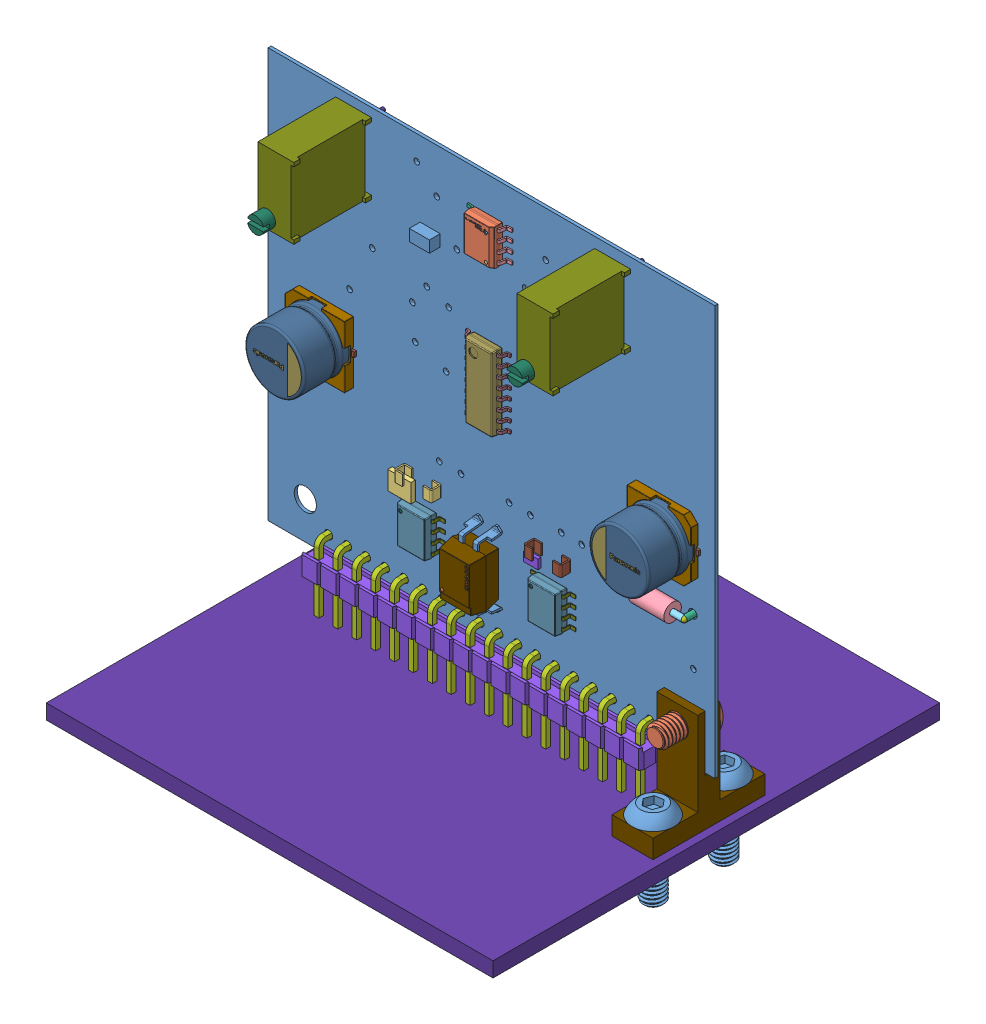
SolidWorks assembly Макет PWM, configuration Default. Lengths in mm. (continued)
Components (placement in the parent): (continued)
- PWM_controller-1: PWM_controller [Default] at (-319.0135 -82.8288 51.7656) size (60 62.62 16.05) (continued)
  - PWM_controller.step-1: PWM_controller.step [Default] at origin size (60 62.62 16.05) (continued)
    - C7.step-1: C7.step [Default] at origin size (1.25 2 0.88) (continued)
      - Cap_KEMET_C0805C472J3HAC_eec-3.step-1: Cap_KEMET_C0805C472J3HAC_eec-3.step [Default] at (216.662 76.6318 -0.4115) x (0 -1 0) z (0 0 -1) size (2 1.25 0.88)
      - Cap_KEMET_C0805C472J3HAC_eec-4.step-1: Cap_KEMET_C0805C472J3HAC_eec-4.step [Default] at (216.662 76.6318 -0.4115) x (0 -1 0) z (0 0 -1) size (0.59 0.12 0)
    - R14.step-1: R14.step [Default] at origin size (2.5 3.2 0.6)
      - Res_Vishay_CRCW12104K70FKEC_eec.step-1: Res_Vishay_CRCW12104K70FKEC_eec.step [Default] at (209.55 54.0512 -0.4115) x (0 -1 0) z (0 0 -1) size (3.2 2.5 0.6)
        - body-11.step-1: body-11.step [Default] at (0 0 0.55) x (1 0 0) z (0 0 -1) size (3.1 2.5 0.5)
        - pad-12.step-1: pad-12.step [Default] at (-1.4133 -1.25 0.6) x (1 0 0) z (0 1 0) size (0.45 0.6 2.5)
        - pad-12.step-2: pad-12.step [Default] at (1.4133 1.25 0.6) x (-1 0 0) z (0 -1 0) size (0.45 0.6 2.5)
        - top-13.step-1: top-13.step [Default] at (0 0 0.6) x (1 0 0) z (0 0 -1) size (2.4 2.5 0.05)
        - Vishay-14.step-1: Vishay-14.step [Default] at (0.0049 -0.739 0.6) size (0.44 0.37 0)
        - bottom.step-1: bottom.step [Default] at (0 0 0.05) x (1 0 0) z (0 0 -1) size (2.3 2.5 0.05)
    - R13.step-1: R13.step [Default] at origin size (2.5 3.2 0.6)
      - Res_Vishay_CRCW12104K70FKEC_eec.step-1: Res_Vishay_CRCW12104K70FKEC_eec.step [Default] at (213.2584 54.1274 -0.4115) x (0 -1 0) z (0 0 -1) size (3.2 2.5 0.6)
        - body-11.step-1: body-11.step [Default] at (0 0 0.55) x (1 0 0) z (0 0 -1) size (3.1 2.5 0.5)
        - pad-12.step-1: pad-12.step [Default] at (-1.4133 -1.25 0.6) x (1 0 0) z (0 1 0) size (0.45 0.6 2.5)
        - pad-12.step-2: pad-12.step [Default] at (1.4133 1.25 0.6) x (-1 0 0) z (0 -1 0) size (0.45 0.6 2.5)
        - top-13.step-1: top-13.step [Default] at (0 0 0.6) x (1 0 0) z (0 0 -1) size (2.4 2.5 0.05)
        - Vishay-14.step-1: Vishay-14.step [Default] at (0.0049 -0.739 0.6) size (0.44 0.37 0)
        - bottom.step-1: bottom.step [Default] at (0 0 0.05) x (1 0 0) z (0 0 -1) size (2.3 2.5 0.05)
    - R16.step-1: R16.step [Default] at origin size (2 1.25 0.5)
      - Res_Vishay_CRCW0805100KFKEA_eec.step-1: Res_Vishay_CRCW0805100KFKEA_eec.step [Default] at (208.6004 62.611 -0.4115) x (-1 0 0) z (0 0 -1) size (2 1.25 0.5)
        - body-1.step-1: body-1.step [Default] at (0 0 0.45) x (1 0 0) z (0 0 -1) size (1.9 1.25 0.4)
        - pad.step-1: pad.step [Default] at (-0.8133 -0.625 0.5) x (1 0 0) z (0 1 0) size (0.3 0.5 1.25)
        - pad.step-2: pad.step [Default] at (0.8133 0.625 0.5) x (-1 0 0) z (0 -1 0) size (0.3 0.5 1.25)
        - top-2.step-1: top-2.step [Default] at (0 0 0.05) x (1 0 0) z (0 0 -1) size (1.4 1.25 0.05)
        - top-2.step-2: top-2.step [Default] at (0 0 0.5) x (1 0 0) z (0 0 -1) size (1.4 1.25 0.05)
        - Vishay.step-1: Vishay.step [Default] at (0.032 -0.7832 0.5) size (0.44 0.37 0)
    - R7.step-1: R7.step [Default] at origin size (1.25 2 0.5)
      - Res_Vishay_CRCW0805100KFKEA_eec.step-1: Res_Vishay_CRCW0805100KFKEA_eec.step [Default] at (232.0544 70.231 -0.4115) x (0 1 0) z (0 0 -1) size (2 1.25 0.5)
        - body-1.step-1: body-1.step [Default] at (0 0 0.45) x (1 0 0) z (0 0 -1) size (1.9 1.25 0.4)
        - pad.step-1: pad.step [Default] at (-0.8133 -0.625 0.5) x (1 0 0) z (0 1 0) size (0.3 0.5 1.25)
        - pad.step-2: pad.step [Default] at (0.8133 0.625 0.5) x (-1 0 0) z (0 -1 0) size (0.3 0.5 1.25)
        - top-2.step-1: top-2.step [Default] at (0 0 0.05) x (1 0 0) z (0 0 -1) size (1.4 1.25 0.05)
        - top-2.step-2: top-2.step [Default] at (0 0 0.5) x (1 0 0) z (0 0 -1) size (1.4 1.25 0.05)
        - Vishay.step-1: Vishay.step [Default] at (0.032 -0.7832 0.5) size (0.44 0.37 0)
    - R15.step-1: R15.step [Default] at origin size (2 1.25 0.5)
      - Res_Vishay_CRCW0805100KFKEA_eec.step-1: Res_Vishay_CRCW0805100KFKEA_eec.step [Default] at (208.6102 60.7568 -0.4115) x (-1 0 0) z (0 0 -1) size (2 1.25 0.5)
        - body-1.step-1: body-1.step [Default] at (0 0 0.45) x (1 0 0) z (0 0 -1) size (1.9 1.25 0.4)
        - pad.step-1: pad.step [Default] at (-0.8133 -0.625 0.5) x (1 0 0) z (0 1 0) size (0.3 0.5 1.25)
        - pad.step-2: pad.step [Default] at (0.8133 0.625 0.5) x (-1 0 0) z (0 -1 0) size (0.3 0.5 1.25)
        - top-2.step-1: top-2.step [Default] at (0 0 0.05) x (1 0 0) z (0 0 -1) size (1.4 1.25 0.05)
        - top-2.step-2: top-2.step [Default] at (0 0 0.5) x (1 0 0) z (0 0 -1) size (1.4 1.25 0.05)
        - Vishay.step-1: Vishay.step [Default] at (0.032 -0.7832 0.5) size (0.44 0.37 0)
    - R10.step-1: R10.step [Default] at origin size (1.25 2 0.5)
      - Res_Vishay_CRCW0805100KFKEA_eec.step-1: Res_Vishay_CRCW0805100KFKEA_eec.step [Default] at (229.2096 70.1802 -0.4115) x (0 1 0) z (0 0 -1) size (2 1.25 0.5)
        - body-1.step-1: body-1.step [Default] at (0 0 0.45) x (1 0 0) z (0 0 -1) size (1.9 1.25 0.4)
        - pad.step-1: pad.step [Default] at (-0.8133 -0.625 0.5) x (1 0 0) z (0 1 0) size (0.3 0.5 1.25)
        - pad.step-2: pad.step [Default] at (0.8133 0.625 0.5) x (-1 0 0) z (0 -1 0) size (0.3 0.5 1.25)
        - top-2.step-1: top-2.step [Default] at (0 0 0.05) x (1 0 0) z (0 0 -1) size (1.4 1.25 0.05)
        - top-2.step-2: top-2.step [Default] at (0 0 0.5) x (1 0 0) z (0 0 -1) size (1.4 1.25 0.05)
        - Vishay.step-1: Vishay.step [Default] at (0.032 -0.7832 0.5) size (0.44 0.37 0)
    - R11.step-1: R11.step [Default] at origin size (2.5 3.2 0.6)
      - Res_Vishay_CRCW12104K70FKEC_eec.step-1: Res_Vishay_CRCW12104K70FKEC_eec.step [Default] at (219.4814 54.1528 -0.4115) x (0 -1 0) z (0 0 -1) size (3.2 2.5 0.6)
        - body-11.step-1: body-11.step [Default] at (0 0 0.55) x (1 0 0) z (0 0 -1) size (3.1 2.5 0.5)
        - pad-12.step-1: pad-12.step [Default] at (-1.4133 -1.25 0.6) x (1 0 0) z (0 1 0) size (0.45 0.6 2.5)
        - pad-12.step-2: pad-12.step [Default] at (1.4133 1.25 0.6) x (-1 0 0) z (0 -1 0) size (0.45 0.6 2.5)
        - top-13.step-1: top-13.step [Default] at (0 0 0.6) x (1 0 0) z (0 0 -1) size (2.4 2.5 0.05)
        - Vishay-14.step-1: Vishay-14.step [Default] at (0.0049 -0.739 0.6) size (0.44 0.37 0)
        - bottom.step-1: bottom.step [Default] at (0 0 0.05) x (1 0 0) z (0 0 -1) size (2.3 2.5 0.05)
    - R12.step-1: R12.step [Default] at origin size (1.25 2 0.5)
      - Res_Vishay_CRCW0805100KFKEA_eec.step-1: Res_Vishay_CRCW0805100KFKEA_eec.step [Default] at (218.6686 76.7842 -0.4115) x (0 -1 0) z (0 0 -1) size (2 1.25 0.5)
        - body-1.step-1: body-1.step [Default] at (0 0 0.45) x (1 0 0) z (0 0 -1) size (1.9 1.25 0.4)
        - pad.step-1: pad.step [Default] at (-0.8133 -0.625 0.5) x (1 0 0) z (0 1 0) size (0.3 0.5 1.25)
        - pad.step-2: pad.step [Default] at (0.8133 0.625 0.5) x (-1 0 0) z (0 -1 0) size (0.3 0.5 1.25)
        - top-2.step-1: top-2.step [Default] at (0 0 0.05) x (1 0 0) z (0 0 -1) size (1.4 1.25 0.05)
        - top-2.step-2: top-2.step [Default] at (0 0 0.5) x (1 0 0) z (0 0 -1) size (1.4 1.25 0.05)
        - Vishay.step-1: Vishay.step [Default] at (0.032 -0.7832 0.5) size (0.44 0.37 0)
    - R8.step-1: R8.step [Default] at origin size (2.5 3.2 0.6)
      - Res_Vishay_CRCW12104K70FKEC_eec.step-1: Res_Vishay_CRCW12104K70FKEC_eec.step [Default] at (222.9866 54.1782 -0.4115) x (0 -1 0) z (0 0 -1) size (3.2 2.5 0.6)
        - body-11.step-1: body-11.step [Default] at (0 0 0.55) x (1 0 0) z (0 0 -1) size (3.1 2.5 0.5)
        - pad-12.step-1: pad-12.step [Default] at (-1.4133 -1.25 0.6) x (1 0 0) z (0 1 0) size (0.45 0.6 2.5)
        - pad-12.step-2: pad-12.step [Default] at (1.4133 1.25 0.6) x (-1 0 0) z (0 -1 0) size (0.45 0.6 2.5)
        - top-13.step-1: top-13.step [Default] at (0 0 0.6) x (1 0 0) z (0 0 -1) size (2.4 2.5 0.05)
        - Vishay-14.step-1: Vishay-14.step [Default] at (0.0049 -0.739 0.6) size (0.44 0.37 0)
        - bottom.step-1: bottom.step [Default] at (0 0 0.05) x (1 0 0) z (0 0 -1) size (2.3 2.5 0.05)
    - Q1.step-1: Q1.step [Default] at origin size (4.58 10 4.6)
      - Trans_SHARP_PC817XNNIP0F_eec.step-1: Trans_SHARP_PC817XNNIP0F_eec.step [Default] at (226.441 58.547 0) x (0 1 0) z (0 0 1) size (10 4.58 4.6)
        - body-15.step-1: body-15.step [Default] at origin size (6.5 4.58 4)
        - terminals-16.step-1: terminals-16.step [Default] at origin size (10 3.74 2.73)
        - logo-17.step-1: logo-17.step [Default] at (-3.25 0 4.6) size (4.76 3.7 0)
    - D3.step-1: D3.step [Default] at origin size (6.37 3.44 1.43)
      - 6010098432.step-1: 6010098432.step [Default] at (217.678 63.754 0) size (6.37 3.44 1.43)
        - body.step-1: body.step [Default] at (-2.3 -1.46 0.25) size (3.1 2.5 0.6)
        - Lead.step-1: Lead.step [Default] at (1.38 0 0) size (1.14 1.45 1.43)
        - Lead.step-2: Lead.step [Default] at (-1.38 0 0) x (-1 0 0) z (0 0 1) size (1.14 1.45 1.43)
    - D2.step-1: D2.step [Default] at origin size (8.58 2.35 4.35)
      - 5955066400.step-1: 5955066400.step [Default] at (247.6485 66.3194 1.175) x (0 0 -1) z (1 0 0) size (2.35 2.35 4.7)
        - Cylinder.step-1: Cylinder.step [Default] at origin size (2.35 2.35 4.7)
      - 5955067280.step-1: 5955067280.step [Default] at (252.348 66.3194 1.175) x (0 0 -1) z (1 0 0) size (0.79 0.79 1.55)
        - Cylinder-18.step-1: Cylinder-18.step [Default] at origin size (0.79 0.79 1.55)
      - 5955066240.step-1: 5955066240.step [Default] at (253.8982 66.3196 -2) x (1 0 0) z (0 0 1) size (0.79 0.79 3.17)
        - Cylinder-19.step-1: Cylinder-19.step [Default] at origin size (0.79 0.79 3.17)
      - 5955066160.step-1: 5955066160.step [Default] at (253.8981 66.3195 1.175) x (1 0 0) z (0 0 1) size (0.79 0.79 0.79)
        - Sphere.step-1: Sphere.step [Default] at origin size (0.79 0.79 0.79)
      - 5955066080.step-1: 5955066080.step [Default] at (246.099 66.3195 1.175) x (-1 0 0) z (0 0 1) size (0.79 0.79 0.79)
        - Sphere-20.step-1: Sphere-20.step [Default] at origin size (0.79 0.79 0.79)
      - 5955066000.step-1: 5955066000.step [Default] at (246.0989 66.3196 -2) x (-1 0 0) z (0 0 1) size (0.79 0.79 3.17)
        - Cylinder-21.step-1: Cylinder-21.step [Default] at origin size (0.79 0.79 3.17)
      - 5955065920.step-1: 5955065920.step [Default] at (247.6491 66.3194 1.175) x (0 0 -1) z (-1 0 0) size (0.79 0.79 1.55)
        - Cylinder-22.step-1: Cylinder-22.step [Default] at origin size (0.79 0.79 1.55)
    - D1.step-1: D1.step [Default] at origin size (5.77 2.81 1.43)
      - 6702799872.step-1: 6702799872.step [Default] at (235.077 63.754 0) x (1 0 0) z (0 0 1) size (5.77 2.81 1.43)
        - body-1.step-1: body-1.step [Default] at (-2.3 -1.46 0.25) size (1.9 1.25 0.4)
        - Lead-24.step-1: Lead-24.step [Default] at (1.38 0 0) size (1.14 1.45 1.43)
        - Lead-24.step-2: Lead-24.step [Default] at (-1.38 0 0) x (-1 0 0) z (0 0 1) size (1.14 1.45 1.43)
    - C8.step-1: C8.step [Default] at origin size (2.7 3.4 1)
      - 6948496496.step-1: 6948496496.step [Default] at (233.2228 57.986 -1.4115) size (2.7 0.5 1)
        - Extruded.step-1: Extruded.step [Default] at origin size (2.7 0.5 1)
      - 6948496496.step-2: 6948496496.step [Default] at (233.2228 60.886 -1.4115) size (2.7 0.5 1)
        - Extruded.step-1: Extruded.step [Default] at origin size (2.7 0.5 1)
      - 6948486416.step-1: 6948486416.step [Default] at (233.2228 59.436 -1.4115) size (2.7 2.4 1)
        - Extruded-0.step-1: Extruded-0.step [Default] at origin size (2.7 2.4 1)
    - C9.step-1: C9.step [Default] at origin size (2.7 3.4 1)
      - 6948496496.step-1: 6948496496.step [Default] at (216.154 58.9512 -1.4115) size (2.7 0.5 1)
        - Extruded.step-1: Extruded.step [Default] at origin size (2.7 0.5 1)
      - 6948496496.step-2: 6948496496.step [Default] at (216.154 61.8512 -1.4115) size (2.7 0.5 1)
        - Extruded.step-1: Extruded.step [Default] at origin size (2.7 0.5 1)
      - 6948486416.step-1: 6948486416.step [Default] at (216.154 60.4012 -1.4115) size (2.7 2.4 1)
        - Extruded-0.step-1: Extruded-0.step [Default] at origin size (2.7 2.4 1)
    - C10.step-1: C10.step [Default] at origin size (9 8.3 6.5)
      - Cap_Panasonic_Electronic_Components_EEE-FK1H101GP_eec.step-1: Cap_Panasonic_Electronic_Components_EEE-FK1H101GP_eec.step [Default] at (250.45 73.9902 0) x (1 0 0) z (0 0 1) size (9 8.3 6.5)
        - base.step-1: base.step [Default] at origin size (8.3 8.3 1.25)
        - cap.step-1: cap.step [Default] at origin size (8 8 6)
        - pins.step-1: pins.step [Default] at origin size (9 0.65 0.3)
        - logo-10.step-1: logo-10.step [Default] at (0 0 6.5) size (6.48 6.34 0)
    - U1.step-1: U1.step [Default] at origin size (5.99 9.91 1.6)
      - SOIC-16akaD0016AakaM16A.step-1: SOIC-16akaD0016AakaM16A.step [Default] at (226.5679 79.7559 0.97) x (0 -1 0) z (-1 0 0) size (9.91 1.6 5.99)
        - M16A_ASM_24_ASM.step-1: M16A_ASM_24_ASM.step [Default] at origin size (9.91 1.6 5.99)
          - BODY_M16A_17.step-1: BODY_M16A_17.step [Default] at origin size (9.91 1.45 3.92)
          - LEAD_M16A_42.step-1: LEAD_M16A_42.step [Default] at (4.445 -0.6223 2.348) size (0.37 0.98 1.04)
          - LEAD_M16A_42.step-2: LEAD_M16A_42.step [Default] at (3.175 -0.6223 2.348) size (0.37 0.98 1.04)
          - LEAD_M16A_42.step-3: LEAD_M16A_42.step [Default] at (1.905 -0.6223 2.348) size (0.37 0.98 1.04)
          - LEAD_M16A_42.step-4: LEAD_M16A_42.step [Default] at (0.635 -0.6223 2.348) size (0.37 0.98 1.04)
          - LEAD_M16A_42.step-5: LEAD_M16A_42.step [Default] at (-0.635 -0.6223 2.348) size (0.37 0.98 1.04)
          - LEAD_M16A_42.step-6: LEAD_M16A_42.step [Default] at (-1.905 -0.6223 2.348) size (0.37 0.98 1.04)
          - LEAD_M16A_42.step-7: LEAD_M16A_42.step [Default] at (-3.175 -0.6223 2.348) size (0.37 0.98 1.04)
          - LEAD_M16A_42.step-8: LEAD_M16A_42.step [Default] at (-4.445 -0.6223 2.348) size (0.37 0.98 1.04)
          - LEAD_M16A_42.step-9: LEAD_M16A_42.step [Default] at (4.445 -0.6223 -2.348) x (-1 0 0) z (0 0 -1) size (0.37 0.98 1.04)
          - LEAD_M16A_42.step-10: LEAD_M16A_42.step [Default] at (3.175 -0.6223 -2.348) x (-1 0 0) z (0 0 -1) size (0.37 0.98 1.04)
          - LEAD_M16A_42.step-11: LEAD_M16A_42.step [Default] at (1.905 -0.6223 -2.348) x (-1 0 0) z (0 0 -1) size (0.37 0.98 1.04)
          - LEAD_M16A_42.step-12: LEAD_M16A_42.step [Default] at (0.635 -0.6223 -2.348) x (-1 0 0) z (0 0 -1) size (0.37 0.98 1.04)
          - LEAD_M16A_42.step-13: LEAD_M16A_42.step [Default] at (-0.635 -0.6223 -2.348) x (-1 0 0) z (0 0 -1) size (0.37 0.98 1.04)
          - LEAD_M16A_42.step-14: LEAD_M16A_42.step [Default] at (-1.905 -0.6223 -2.348) x (-1 0 0) z (0 0 -1) size (0.37 0.98 1.04)
          - LEAD_M16A_42.step-15: LEAD_M16A_42.step [Default] at (-3.175 -0.6223 -2.348) x (-1 0 0) z (0 0 -1) size (0.37 0.98 1.04)
          - LEAD_M16A_42.step-16: LEAD_M16A_42.step [Default] at (-4.445 -0.6223 -2.348) x (-1 0 0) z (0 0 -1) size (0.37 0.98 1.04)
    - U2.step-1: U2.step [Default] at origin size (6 5.01 1.75)
      - 6010097792.step-1: 6010097792.step [Default] at (235.204 58.547 0) size (6 5 1.75)
        - Body-2.step-1: Body-2.step [Default] at (-2 -2.5 0) size (4 5 1.65)
          - Open_CASCADE_STEP_translator_6.8_3.2.1.step-1: Open_CASCADE_STEP_translator_6.8_3.2.1.step [Default] at origin size (4 5 1.65)
        - Open_CASCADE_STEP_translator_6.8_3.1.step-1: Open_CASCADE_STEP_translator_6.8_3.1.step [Default] at (-2 -2.5 0.001) size (0.51 0.51 0.01)
        - Leader.step-1: Leader.step [Default] at (-2 -1.905 0) x (-1 0 0) z (0 0 1) size (1 0.42 0.97)
        - Leader.step-2: Leader.step [Default] at (-2 -0.635 0) x (-1 0 0) z (0 0 1) size (1 0.42 0.97)
        - Leader.step-3: Leader.step [Default] at (-2 0.635 0) x (-1 0 0) z (0 0 1) size (1 0.42 0.97)
        - Leader.step-4: Leader.step [Default] at (-2 1.905 0) x (-1 0 0) z (0 0 1) size (1 0.42 0.97)
        - Leader.step-5: Leader.step [Default] at (2 -1.905 0) size (1 0.42 0.97)
        - Leader.step-6: Leader.step [Default] at (2 -0.635 0) size (1 0.42 0.97)
        - Leader.step-7: Leader.step [Default] at (2 0.635 0) size (1 0.42 0.97)
        - Leader.step-8: Leader.step [Default] at (2 1.905 0) size (1 0.42 0.97)
    - U3.step-1: U3.step [Default] at origin size (6 5.01 1.75)
      - 6010097792.step-1: 6010097792.step [Default] at (217.678 58.547 0) size (6 5 1.75)
        - Body-2.step-1: Body-2.step [Default] at (-2 -2.5 0) size (4 5 1.65)
          - Open_CASCADE_STEP_translator_6.8_3.2.1.step-1: Open_CASCADE_STEP_translator_6.8_3.2.1.step [Default] at origin size (4 5 1.65)
        - Open_CASCADE_STEP_translator_6.8_3.1.step-1: Open_CASCADE_STEP_translator_6.8_3.1.step [Default] at (-2 -2.5 0.001) size (0.51 0.51 0.01)
        - Leader.step-1: Leader.step [Default] at (-2 -1.905 0) x (-1 0 0) z (0 0 1) size (1 0.42 0.97)
        - Leader.step-2: Leader.step [Default] at (-2 -0.635 0) x (-1 0 0) z (0 0 1) size (1 0.42 0.97)
        - Leader.step-3: Leader.step [Default] at (-2 0.635 0) x (-1 0 0) z (0 0 1) size (1 0.42 0.97)
        - Leader.step-4: Leader.step [Default] at (-2 1.905 0) x (-1 0 0) z (0 0 1) size (1 0.42 0.97)
        - Leader.step-5: Leader.step [Default] at (2 -1.905 0) size (1 0.42 0.97)
        - Leader.step-6: Leader.step [Default] at (2 -0.635 0) size (1 0.42 0.97)
        - Leader.step-7: Leader.step [Default] at (2 0.635 0) size (1 0.42 0.97)
        - Leader.step-8: Leader.step [Default] at (2 1.905 0) size (1 0.42 0.97)
- Макет платы-1: Макет платы [Default] at (-92.1635 -41.4968 51.5599) size (60 2 60)
- Кронштейн под плату PWM Controller, сборка-1: Кронштейн под плату PWM Controller, сборка [Default] at origin size (6.69 22.28 16.09)
  - Кронштейн под плату PWM Controller-1: Кронштейн под плату PWM Controller [Default] at (-65.9135 -34.1968 51.5599) size (5.5 13.8 15)
  - Винт M3-1: Винт M3 [Default] at (-65.9135 -39.2651 46.8099) x (0.981349 0 -0.192232) z (0.192232 0 0.981349) size (5.6 11.53 5.6)
  - Винт M3х6-1: Винт M3х6 [Default] at (-65.9135 -29.1968 51.3282) x (-0.218761 0.975778 0) z (-0.975778 -0.218761 0) size (5.6 7.51 5.6)
  - Винт M3-2: Винт M3 [Default] at (-65.9135 -39.2651 56.3099) x (0.979315 0 -0.202341) z (0.202341 0 0.979315) size (5.6 11.53 5.6)
Mates (geometry in assembly coordinates):
- Distance1: distance = 6.3 mm anti-aligned: plane of Макет платы-1 through (-92.1635 -40.4968 51.5599) normal (0 1 0); plane of PWM_controller-1/PWM_controller.step-1/Board.step-1/Open CASCADE STEP translator 6.8 2.1.1.step-1 through (-62.1635 -34.1968 51.3542) normal (0 -1 0)
- Width1: width aligned: plane of Макет платы-1 through (-122.1635 -40.4968 81.5599) normal (0 0 1); plane of PWM_controller-1/PWM_controller.step-1/Board.step-1/Open CASCADE STEP translator 6.8 2.1.1.step-1 through (-122.1635 -40.4968 21.5599) normal (0 0 -1); plane of Макет платы-1 through (-122.1635 -34.1968 51.7656) normal (0 0 1); plane of PWM_controller-1/PWM_controller.step-1/Board.step-1/Open CASCADE STEP translator 6.8 2.1.1.step-1 through (-122.1635 -34.1968 51.3542) normal (0 0 -1)
- Width2: width aligned: plane of PWM_controller-1/PWM_controller.step-1/Board.step-1/Open CASCADE STEP translator 6.8 2.1.1.step-1 through (-122.1635 -34.1968 51.3542) normal (-1 0 0); plane of Макет платы-1 through (-62.1635 20.8032 51.3542) normal (1 0 0); plane of PWM_controller-1/PWM_controller.step-1/Board.step-1/Open CASCADE STEP translator 6.8 2.1.1.step-1 through (-122.1635 -40.4968 21.5599) normal (-1 0 0); plane of Макет платы-1 through (-62.1635 -40.4968 21.5599) normal (1 0 0)
- Coincident6: coincident anti-aligned: plane of Макет платы-1 through (-92.1635 -40.4968 51.5599) normal (0 1 0); plane of Кронштейн под плату PWM Controller, сборка-1/Кронштейн под плату PWM Controller-1 through (-63.1635 -40.4968 59.0599) normal (0 -1 0)
- Width4: width anti-aligned: plane of Кронштейн под плату PWM Controller, сборка-1/Кронштейн под плату PWM Controller-1 through (-63.1635 -26.6968 52.0599) normal (0 0 -1); plane of PWM_controller-1/PWM_controller.step-1/Board.step-1/Open CASCADE STEP translator 6.8 2.1.1.step-1 through (-63.1635 -26.6968 51.0599) normal (0 0 1); plane of Кронштейн под плату PWM Controller, сборка-1/Кронштейн под плату PWM Controller-1 through (-122.1635 -34.1968 51.7656) normal (0 0 1); plane of PWM_controller-1/PWM_controller.step-1/Board.step-1/Open CASCADE STEP translator 6.8 2.1.1.step-1 through (-122.1635 -34.1968 51.3542) normal (0 0 -1)
- Distance3: distance = 1 mm aligned: plane of Кронштейн под плату PWM Controller, сборка-1/Кронштейн под плату PWM Controller-1 through (-63.1635 -34.1968 51.5599) normal (1 0 0); plane of PWM_controller-1/PWM_controller.step-1/Board.step-1/Open CASCADE STEP translator 6.8 2.1.1.step-1 through (-62.1635 20.8032 51.3542) normal (1 0 0)
